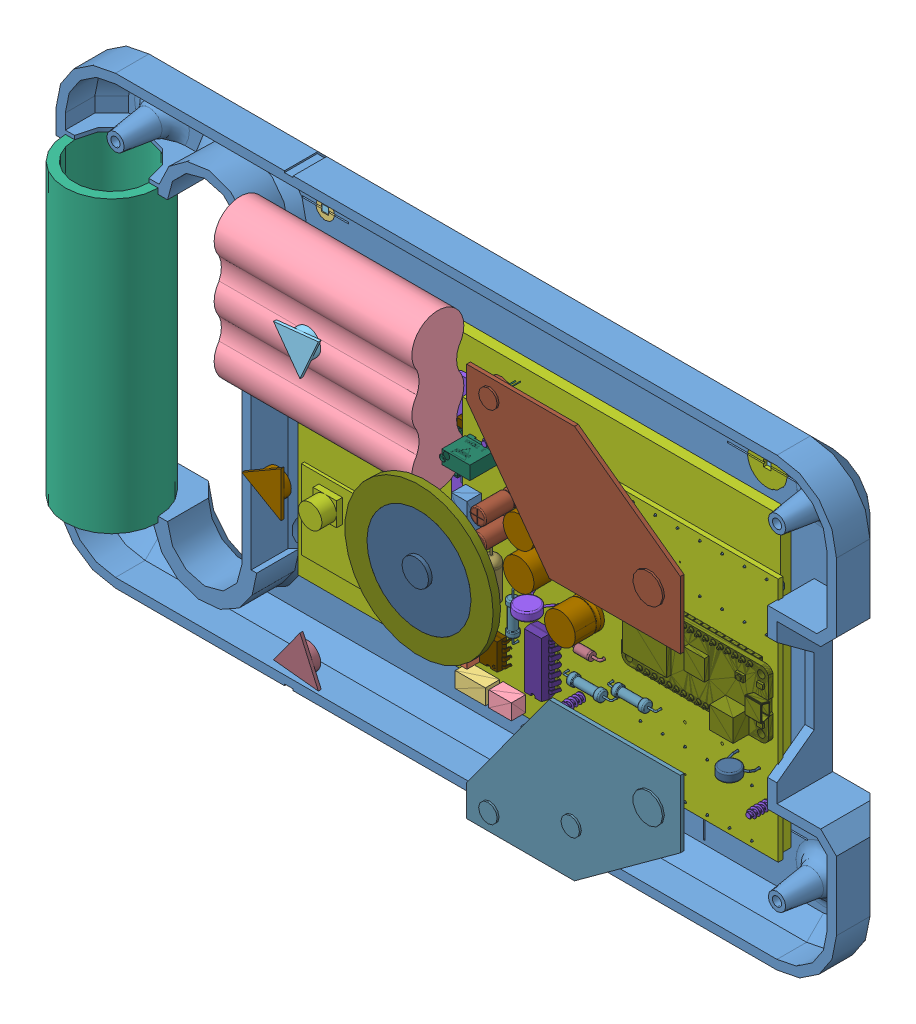
SolidWorks assembly sheikah assembled, configuration Default. Lengths in mm.
Overall size (266.7 152.4 43.32).
174 component instances, 63 part files, 41 mates.
Components (placement in the parent):
- Sheikah Slate Body Converted Assembly-1: Sheikah Slate Body Converted Assembly [Default] at origin size (273.52 152.4 41.91)
  - Front Body-1: Front Body [Default] at origin size (266.7 152.4 21.73)
  - Bottom Right Disk-1: Bottom Right Disk [Default] at origin size (9.21 9.21 0.64)
  - Top Right Blue LED Holder-1: Top Right Blue LED Holder [Default] at origin size (6.31 6.31 3.81)
  - Top Left Disk-1: Top Left Disk [Default] at origin size (7.69 7.69 0.64)
  - Eyelash Orange LED1-1: Eyelash Orange LED1 [Default] at origin size (15.32 14.07 3.54)
  - Handle Tube-1: Handle Tube [Default] at origin size (31.75 99.06 31.75)
  - Top Left Blue LED Holder-2: Top Left Blue LED Holder [Default] at origin size (13.47 13.47 3.81)
  - Bottom Right Blue LED Holder-1: Bottom Right Blue LED Holder [Default] at origin size (14.66 14.66 3.81)
  - Eyelash Orange LED2-3: Eyelash Orange LED2 [Default] at origin size (13.36 15.4 3.54)
  - Inner Neopixel Ring Holder-1: Inner Neopixel Ring Holder [Default] at origin size (35.56 35.56 3.81)
  - Left Orange LED Panel-1: Left Orange LED Panel [Default] at origin size (73.01 49.3 4.45)
  - Bottom Middle Blue LED Holder-1: Bottom Middle Blue LED Holder [Default] at origin size (10.16 10.16 3.81)
  - Eyelash Orange LED3-2: Eyelash Orange LED3 [Default] at origin size (15.32 14.07 3.54)
  - Right Orange LED Panel-1: Right Orange LED Panel [Default] at origin size (73.01 49.3 4.45)
  - Bottom Left Blue LED Holder-1: Bottom Left Blue LED Holder [Default] at origin size (11.44 11.44 3.81)
  - Outer Neopixel Ring Holder-1: Outer Neopixel Ring Holder [Default] at origin size (50.68 50.68 2.54)
  - Back Body-1: Back Body [Default] at origin size (273.52 152.4 34.3) (hidden)
- Neopixel Jewel RGBW-1: Neopixel Jewel RGBW [Default] at (92.2855 47.625 14.545) size (23 23 3.23)
  - Neopixel Jewel RGBW.stp-1: Neopixel Jewel RGBW.stp [Default] at origin size (23 23 3.23)
    - WS2812B-NARROW.stp-1: WS2812B-NARROW.stp [Default] at (0 0 1.6) x (0 -1 0) z (0 0 1) size (5 5.45 1.68)
      - body.stp-1: body.stp [Default] at origin size (5 5 1.6)
      - leads.stp-1: leads.stp [Default] at origin size (4.2 5.45 0.88)
      - processor.stp-1: processor.stp [Default] at origin size (0.8 0.6 0.1)
      - lense.stp-1: lense.stp [Default] at origin size (4 4 0.39)
    - WS2812B-NARROW_1.stp-1: WS2812B-NARROW_1.stp [Default] at (6.9 4 1.6) x (-0.866025 -0.5 0) z (0 0 1) size (5 5.45 1.68)
      - body.stp-1: body.stp [Default] at origin size (5 5 1.6)
      - leads.stp-1: leads.stp [Default] at origin size (4.2 5.45 0.88)
      - processor.stp-1: processor.stp [Default] at origin size (0.8 0.6 0.1)
      - lense.stp-1: lense.stp [Default] at origin size (4 4 0.39)
    - WS2812B-NARROW_2.stp-1: WS2812B-NARROW_2.stp [Default] at (-6.9 4 1.6) x (0.866025 -0.5 0) z (0 0 1) size (5 5.45 1.68)
      - body.stp-1: body.stp [Default] at origin size (5 5 1.6)
      - leads.stp-1: leads.stp [Default] at origin size (4.2 5.45 0.88)
      - processor.stp-1: processor.stp [Default] at origin size (0.8 0.6 0.1)
      - lense.stp-1: lense.stp [Default] at origin size (4 4 0.39)
    - WS2812B-NARROW_3.stp-1: WS2812B-NARROW_3.stp [Default] at (-6.9 -4 1.6) x (0.866025 0.5 0) z (0 0 1) size (5 5.45 1.68)
      - body.stp-1: body.stp [Default] at origin size (5 5 1.6)
      - leads.stp-1: leads.stp [Default] at origin size (4.2 5.45 0.88)
      - processor.stp-1: processor.stp [Default] at origin size (0.8 0.6 0.1)
      - lense.stp-1: lense.stp [Default] at origin size (4 4 0.39)
    - WS2812B-NARROW_4.stp-1: WS2812B-NARROW_4.stp [Default] at (0 8 1.6) x (0 -1 0) z (0 0 1) size (5 5.45 1.68)
      - body.stp-1: body.stp [Default] at origin size (5 5 1.6)
      - leads.stp-1: leads.stp [Default] at origin size (4.2 5.45 0.88)
      - processor.stp-1: processor.stp [Default] at origin size (0.8 0.6 0.1)
      - lense.stp-1: lense.stp [Default] at origin size (4 4 0.39)
    - WS2812B-NARROW_5.stp-1: WS2812B-NARROW_5.stp [Default] at (6.9 -4 1.6) x (-0.866025 0.5 0) z (0 0 1) size (5 5.45 1.68)
      - body.stp-1: body.stp [Default] at origin size (5 5 1.6)
      - leads.stp-1: leads.stp [Default] at origin size (4.2 5.45 0.88)
      - processor.stp-1: processor.stp [Default] at origin size (0.8 0.6 0.1)
      - lense.stp-1: lense.stp [Default] at origin size (4 4 0.39)
    - WS2812B-NARROW_6.stp-1: WS2812B-NARROW_6.stp [Default] at (0 -8.2 1.6) x (0 1 0) z (0 0 1) size (5 5.45 1.68)
      - body.stp-1: body.stp [Default] at origin size (5 5 1.6)
      - leads.stp-1: leads.stp [Default] at origin size (4.2 5.45 0.88)
      - processor.stp-1: processor.stp [Default] at origin size (0.8 0.6 0.1)
      - lense.stp-1: lense.stp [Default] at origin size (4 4 0.39)
    - pcb.stp-1: pcb.stp [Default] at origin size (23 23 1.6)
    - C0603.stp-1: C0603.stp [Default] at (-4.7192 -8.094 1.6) x (-0.5 -0.866025 0) z (0 0 1) size (2.33 0.91 0.82)
    - C0603.stp-2: C0603.stp [Default] at (-4.6 8.1 1.6) x (-0.5 0.866025 0) z (0 0 1) size (2.33 0.91 0.82)
    - C0603.stp-3: C0603.stp [Default] at (4.9743 8.1743 1.6) x (0.707107 0.707107 0) z (0 0 1) size (2.33 0.91 0.82)
    - C0603.stp-4: C0603.stp [Default] at (4.694 -8.0316 1.6) x (0.5 -0.866025 0) z (0 0 1) size (2.33 0.91 0.82)
    - R0603-NO.stp-1: R0603-NO.stp [Default] at (-4.2552 0.1809 1.6) x (0 1 0) z (0 0 1) size (2.31 0.91 0.45)
- NeoPixelRing16-1: NeoPixelRing16 [Default] at (92.2855 47.625 15.58) x (0.587442 0.809266 0) z (0 0 1) size (44 44 2.55)
- HDMI 7po adafruit-2: HDMI 7po adafruit [Défaut] at (101.9311 44.1111 -8.025) x (-1 0 0) z (0 0 -1) size (164.95 100 3.45)
- Adafruit RA8875 TFT Breakout-1: Adafruit RA8875 TFT Breakout [Default] at (73.4911 41.9804 -12.425) size (48.26 40.64 4.01)
  - Adafruit RA8875 TFT Breakout.step-1: Adafruit RA8875 TFT Breakout.step [Default] at origin size (48.26 40.64 4.01)
    - PCB Component.step-1: PCB Component.step [Default] at origin size (48.26 40.64 4.01)
      - Board.step-1: Board.step [Default] at origin size (48.26 40.64 1.57)
      - RA8875.step-1: RA8875.step [Default] at (25.646 17.018 1.57) size (16 16 1.6)
      - 10K.step-1: 10K.step [Default] at (14.47 28.702 1.57) x (-1 0 0) z (0 0 1) size (2 1.25 1)
      - 10K.step-2: 10K.step [Default] at (10.406 11.684 1.57) x (0 1 0) z (0 0 1) size (2 1.25 1)
      - 10K.step-3: 10K.step [Default] at (9.644 14.732 1.57) size (2 1.25 1)
      - 10K.step-4: 10K.step [Default] at (13.581 10.668 1.57) x (-1 0 0) z (0 0 1) size (2 1.25 1)
      - 10K.step-5: 10K.step [Default] at (13.962 20.955 1.57) x (-1 0 0) z (0 0 1) size (2 1.25 1)
      - 10K.step-6: 10K.step [Default] at (36.822 17.272 1.57) size (2 1.25 1)
      - 10K.step-7: 10K.step [Default] at (34.917 9.652 1.57) size (2 1.25 1)
      - 10K.step-8: 10K.step [Default] at (16.248 8.382 1.57) x (-1 0 0) z (0 0 1) size (2 1.25 1)
      - 10K.step-9: 10K.step [Default] at (37.33 23.241 1.57) x (0 -1 0) z (0 0 1) size (2 1.25 1)
      - 10K.step-10: 10K.step [Default] at (12.438 8.382 1.57) x (-1 0 0) z (0 0 1) size (2 1.25 1)
      - 10K.step-11: 10K.step [Default] at (13.962 19.05 1.57) x (-1 0 0) z (0 0 1) size (2 1.25 1)
      - 10K.step-12: 10K.step [Default] at (13.962 17.272 1.57) x (-1 0 0) z (0 0 1) size (2 1.25 1)
      - 10K.step-13: 10K.step [Default] at (36.822 15.113 1.57) size (2 1.25 1)
      - 10K.step-14: 10K.step [Default] at (38.981 10.414 1.57) x (0 1 0) z (0 0 1) size (2 1.25 1)
      - 20MHz.step-1: 20MHz.step [Default] at (13.454 13.716 1.57) x (0 1 0) z (0 0 1) size (3.8 3 0.4)
      - 33.step-1: 33.step [Default] at (31.996 29.21 1.57) size (3.05 1.6 0.5)
      - 33.step-2: 33.step [Default] at (28.186 29.21 1.57) size (3.05 1.6 0.5)
      - 33.step-3: 33.step [Default] at (24.376 29.21 1.57) size (3.05 1.6 0.5)
      - 33.step-4: 33.step [Default] at (20.566 29.21 1.57) size (3.05 1.6 0.5)
      - 33.step-5: 33.step [Default] at (35.806 29.21 1.57) size (3.05 1.6 0.5)
      - 40PINFPCM4-1734839-0.step-1: 40PINFPCM4-1734839-0.step [Default] at (28.44 37.592 1.57) size (25.43 5.11 2.05)
      - FAN5333BSX.step-1: FAN5333BSX.step [Default] at (2.786 21.082 1.57) x (-1 0 0) z (0 0 1) size (3 3 1.4)
      - 3Ω.step-1: 3Ω.step [Default] at (6.596 18.034 1.57) size (2 1.25 0.85)
      - 3Ω.step-2: 3Ω.step [Default] at (2.786 24.13 1.57) x (-1 0 0) z (0 0 1) size (2 1.25 0.85)
      - 3Ω.step-3: 3Ω.step [Default] at (12.962 24.638 1.57) x (0 -1 0) z (0 0 1) size (2 1.25 0.85)
      - 3Ω.step-4: 3Ω.step [Default] at (6.731 25.916 1.57) size (2 1.25 0.85)
      - 3Ω.step-5: 3Ω.step [Default] at (2.786 18.034 1.57) size (2 1.25 0.85)
      - 3Ω.step-6: 3Ω.step [Default] at (17.01 29.972 1.57) x (0 -1 0) z (0 0 1) size (2 1.25 0.85)
      - 3Ω.step-7: 3Ω.step [Default] at (2.278 11.43 1.57) x (0 1 0) z (0 0 1) size (2 1.25 0.85)
      - 3Ω.step-8: 3Ω.step [Default] at (15.559 33.198 1.57) x (-1 0 0) z (0 0 1) size (2 1.25 0.85)
      - 3Ω.step-9: 3Ω.step [Default] at (8.628 11.811 1.57) x (0 1 0) z (0 0 1) size (2 1.25 0.85)
      - 3Ω.step-10: 3Ω.step [Default] at (6.723 8.763 1.57) x (-1 0 0) z (0 0 1) size (2 1.25 0.85)
      - 3Ω.step-11: 3Ω.step [Default] at (2.667 25.908 1.57) size (2 1.25 0.85)
      - 3Ω.step-12: 3Ω.step [Default] at (1.27 29.972 1.57) x (0 1 0) z (0 0 1) size (2 1.25 0.85)
      - 6.8uH large inductor.step-1: 6.8uH large inductor.step [Default] at (7.358 21.844 1.57) x (0 1 0) z (0 0 1) size (4 4 1.8)
      - MBR0540.step-1: MBR0540.step [Default] at (11.168 24.511 1.57) x (0 -1 0) z (0 0 1) size (3.6 1.4 1.35)
      - MM3Z24VT1G.step-1: MM3Z24VT1G.step [Default] at (6.215 28.702 1.57) x (-1 0 0) z (0 0 1) size (5.04 2.7 2.44)
      - MIC5225-3.3v.step-1: MIC5225-3.3v.step [Default] at (5.326 11.684 1.57) x (0 1 0) z (0 0 1) size (3 3 1.4)
      - 74HC4050.step-1: 74HC4050.step [Default] at (43.045 19.685 1.57) x (0 -1 0) z (0 0 1) size (10 6.2 1.75)
      - 1N4148.step-1: 1N4148.step [Default] at (5.842 15.113 1.57) size (2.7 1.35 1.1)
      - 1N4148.step-2: 1N4148.step [Default] at (2.54 15.113 1.57) x (-1 0 0) z (0 0 1) size (2.7 1.35 1.1)
- adafruit 5035 battery-1: adafruit 5035 battery [Default] at (52.8771 89.0109 15.875) x (-1 0 0) z (0 0 -1) size (67.56 53.34 17.78)
- HLMP-QB00-S0000-1: HLMP-QB00-S0000 [Default] at (24.6439 5.2882 -17.526) x (-1 0 0) z (0 0 1) size (2.21 2.21 2.79)
- HLMP-QB00-S0000-2: HLMP-QB00-S0000 [Default] at (119.6309 -5.6441 -17.526) x (-1 0 0) z (0 0 1) size (2.21 2.21 2.79)
- HLMP-QB00-S0000-3: HLMP-QB00-S0000 [Default] at (172.4751 -0.773 -17.525) x (-1 0 0) z (0 0 1) size (2.21 2.21 2.79)
- HLMP-QB00-S0000-4: HLMP-QB00-S0000 [Default] at (176.2779 103.3091 -18.542) x (-1 0 0) z (0 0 1) size (2.21 2.21 2.79)
- HLMP-QB00-S0000-5: HLMP-QB00-S0000 [Default] at (25.225 103.4991 -17.526) x (-1 0 0) z (0 0 1) size (2.21 2.21 2.79)
- SLR-343DC3F-1: SLR-343DC3F [Default] at (169.1626 80.1556 11.38) x (-0.923728 -0.383049 0) z (-0.383049 0.923728 0) size (3.8 9.21 3.51)
- SLR-343DC3F-2: SLR-343DC3F [Default] at (114.5671 -13.6866 11.38) x (-0.923728 -0.383049 0) z (-0.383049 0.923728 0) size (3.8 9.21 3.51)
- SLR-343DC3F-3: SLR-343DC3F [Default] at (142.6962 -3.5762 11.38) x (-0.923728 -0.383049 0) z (-0.383049 0.923728 0) size (3.8 9.21 3.51)
- SLR-343DC3F-4: SLR-343DC3F [Default] at (169.1626 15.0944 11.38) x (-0.923728 -0.383049 0) z (-0.383049 0.923728 0) size (3.8 9.21 3.51)
- SLR-343DC3F-6: SLR-343DC3F [Default] at (114.5671 108.9366 11.38) x (-0.923728 -0.383049 0) z (-0.383049 0.923728 0) size (3.8 9.21 3.51)
- MCB-1: MCB [Default] at (101.2945 92.9812 -3.2654) x (0 -1 0) z (0 0 1) size (83.82 111.16 36.76)
  - SHEIKAHSLATE-1: SHEIKAHSLATE [Default] at origin size (83.82 111.16 36.76)
    - Board_SHEIKAHSLATE-1: Board_SHEIKAHSLATE [Default] at origin size (83.82 107.95 1.59)
    - HAU470KBAUARKR-1: HAU470KBAUARKR [Default] at (53.34 12.7 0.05) x (0 1 0) z (0 0 1) size (8 3 13.01)
    - MALREKA00DE433BG0K-1: MALREKA00DE433BG0K [Default] at (50.8 26.83 0.05) x (0 1 0) z (0 0 1) size (10.51 10.5 11.95)
    - MALREKA00DE433BG0K-2: MALREKA00DE433BG0K [Default] at (29.21 12.7 0.05) size (10.51 10.5 11.95)
    - MALREKA00DE433BG0K-3: MALREKA00DE433BG0K [Default] at (41.91 12.7 0.05) size (10.51 10.5 11.95)
    - A102J15C0GF5UAAP-1: A102J15C0GF5UAAP [Default] at (67.31 81.28 0.05) x (0 -1 0) z (0 0 1) size (7.99 3 12.01)
    - Noname_1-1: Noname_1 [Default] at (36.83 1.27 0.05) size (5.5 5.5 14.5)
    - Noname_1-2: Noname_1 [Default] at (29.21 1.27 0.05) size (5.5 5.5 14.5)
    - TVA1161-1: TVA1161 [Default] at (54.61 -3.81 0.05) size (21.4 5.51 7.51)
    - 1N5819G-1: 1N5819G [Default] at (62.23 26.67 0) x (0 -1 0) z (0 0 1) size (11.27 2.71 4.71)
    - Noname_2-1: Noname_2 [Default] at (67.31 43.18 0) x (0 -1 0) z (0 0 1) size (16.91 3.6 5.6)
    - Noname_2-2: Noname_2 [Default] at (46.99 58.42 -1.5896) x (0 1 0) z (0 0 -1) size (16.91 3.6 5.6)
    - Noname_2-3: Noname_2 [Default] at (19.05 87.63 -1.5896) x (-1 0 0) z (0 0 -1) size (16.91 3.6 5.6)
    - Noname_2-4: Noname_2 [Default] at (19.05 80.01 -1.5896) x (-1 0 0) z (0 0 -1) size (16.91 3.6 5.6)
    - Noname_2-5: Noname_2 [Default] at (19.05 72.39 -1.5896) x (-1 0 0) z (0 0 -1) size (16.91 3.6 5.6)
    - Noname_2-6: Noname_2 [Default] at (19.05 64.77 -1.5896) x (-1 0 0) z (0 0 -1) size (16.91 3.6 5.6)
    - Noname_2-7: Noname_2 [Default] at (19.05 57.15 -1.5896) x (-1 0 0) z (0 0 -1) size (16.91 3.6 5.6)
    - Noname_2-8: Noname_2 [Default] at (19.05 49.53 -1.5896) x (-1 0 0) z (0 0 -1) size (16.91 3.6 5.6)
    - Noname_2-9: Noname_2 [Default] at (19.05 41.91 -1.5896) x (-1 0 0) z (0 0 -1) size (16.91 3.6 5.6)
    - Noname_2-10: Noname_2 [Default] at (19.05 34.29 -1.5896) x (-1 0 0) z (0 0 -1) size (16.91 3.6 5.6)
    - Noname_2-11: Noname_2 [Default] at (19.05 26.67 -1.5896) x (-1 0 0) z (0 0 -1) size (16.91 3.6 5.6)
    - Noname_2-12: Noname_2 [Default] at (19.05 19.05 -1.5896) x (-1 0 0) z (0 0 -1) size (16.91 3.6 5.6)
    - Noname_2-13: Noname_2 [Default] at (82.55 44.45 -1.5896) x (1 0 0) z (0 0 -1) size (16.91 3.6 5.6)
    - Noname_2-14: Noname_2 [Default] at (82.55 52.07 -1.5896) x (1 0 0) z (0 0 -1) size (16.91 3.6 5.6)
    - Noname_2-15: Noname_2 [Default] at (82.55 59.69 -1.5896) x (1 0 0) z (0 0 -1) size (16.91 3.6 5.6)
    - Noname_2-16: Noname_2 [Default] at (82.55 67.31 -1.5896) x (1 0 0) z (0 0 -1) size (16.91 3.6 5.6)
    - Noname_2-17: Noname_2 [Default] at (82.55 74.93 -1.5896) x (1 0 0) z (0 0 -1) size (16.91 3.6 5.6)
    - Noname_2-18: Noname_2 [Default] at (82.55 82.55 -1.5896) x (1 0 0) z (0 0 -1) size (16.91 3.6 5.6)
    - Noname_2-19: Noname_2 [Default] at (48.26 78.74 -1.5896) x (0 -1 0) z (0 0 -1) size (16.91 3.6 5.6)
    - Noname_2-20: Noname_2 [Default] at (39.37 78.74 -1.5896) x (0 1 0) z (0 0 -1) size (16.91 3.6 5.6)
    - Noname_2-21: Noname_2 [Default] at (71.755 27.94 0) x (0 1 0) z (0 0 1) size (16.91 3.6 5.6)
    - Noname_2-22: Noname_2 [Default] at (39.37 58.42 -1.5896) x (0 1 0) z (0 0 -1) size (16.91 3.6 5.6)
    - Noname_2-23: Noname_2 [Default] at (63.5 2.54 0) size (16.91 3.6 5.6)
    - T93YA-1: T93YA [Default] at (20.32 -13.69 5) size (12.52 14.14 22.04)
    - Adafruit_Feather_M0_Adalogger-1: Adafruit_Feather_M0_Adalogger [Default] at (45.72 66.04 3) x (0 -1 0) z (0 0 1) size (54.99 41.16 36.76)
    - SN74HC125N-1: SN74HC125N [Default] at (71.24 12.69 0) x (-1 0 0) z (0 1 0) size (19.31 8.27 10.93)
    - DIP8-1: DIP8 [Default] at (76.2 -3.81 0) size (15.36 12.48 12.48)
    - DIP8-2: DIP8 [Default] at (35.77 29 0) x (0 1 0) z (0 0 1) size (15.36 12.48 12.48)
    - 640453-4-1: 640453-4 [Default] at (39.1318 -16.4465 0) size (10.3 5.34 4.91)
    - 1-640453-5-1: 1-640453-5 [Default] at (64.53 -16.4465 0) size (38.24 5.34 4.91)
    - 640453-4-0-1: 640453-4-0 [Default] at (92.6465 -9.1282 0) x (0 1 0) z (0 0 1) size (10.3 5.34 4.91)
    - 640453-3-1: 640453-3 [Default] at (92.6465 1.0303 0) x (-0.000018 1 0) z (0 0 1) size (7.76 5.34 4.91)
    - PPTC021LFBN-RC-1: PPTC021LFBN-RC [Default] at (88.689 15.24 0) x (0 1 0) z (0 0 1) size (5.94 2.66 8.76)
    - PPTC021LFBN-RC-1-1: PPTC021LFBN-RC-1 [Default] at (88.689 24.13 0) x (-0.000018 1 0) z (0 0 1) size (5.94 2.66 8.76)
- adafruit TTL mini camera-1: adafruit TTL mini camera [Default] at (57.6381 41.125 14.59) x (-1 0 0) z (0 0 -1) size (20 27 14)
- 99461A941_Phillips Rounded Head Thread-Forming Screws-1: 99461A941_Phillips Rounded Head Thread-Forming Screws [99461A941] at (-30.48 -8.255 -12.2325) x (-0.923728 -0.383049 0) z (0 0 -1) size (5.3 5.3 10.3)
- 99461A941_Phillips Rounded Head Thread-Forming Screws-2: 99461A941_Phillips Rounded Head Thread-Forming Screws [99461A941] at (195.58 -8.255 -12.2325) x (-0.923728 -0.383049 0) z (0 0 -1) size (5.3 5.3 10.3)
- 99461A941_Phillips Rounded Head Thread-Forming Screws-3: 99461A941_Phillips Rounded Head Thread-Forming Screws [99461A941] at (-30.48 103.505 -12.2325) x (-0.923728 -0.383049 0) z (0 0 -1) size (5.3 5.3 10.3)
- 99461A941_Phillips Rounded Head Thread-Forming Screws-4: 99461A941_Phillips Rounded Head Thread-Forming Screws [99461A941] at (195.58 103.505 -12.2325) x (-0.923728 -0.383049 0) z (0 0 -1) size (5.3 5.3 10.3)
- 99461A941_Phillips Rounded Head Thread-Forming Screws-5: 99461A941_Phillips Rounded Head Thread-Forming Screws [99461A941] at (98.7545 80.2812 -4.6875) x (-0.923728 -0.383049 0) z (0 0 -1) size (5.3 5.3 10.3)
- 99461A941_Phillips Rounded Head Thread-Forming Screws-6: 99461A941_Phillips Rounded Head Thread-Forming Screws [99461A941] at (125.4245 15.5112 -4.6875) x (-0.923728 -0.383049 0) z (0 0 -1) size (5.3 5.3 10.3)
- 99461A941_Phillips Rounded Head Thread-Forming Screws-7: 99461A941_Phillips Rounded Head Thread-Forming Screws [99461A941] at (189.0345 15.5112 -4.6875) x (-0.923728 -0.383049 0) z (0 0 -1) size (5.3 5.3 10.3)
Mates (geometry in assembly coordinates):
- Coincident10: coincident: plane of HDMI 7po adafruit-2 through (184.4061 94.1111 -12.425) normal (0 0 1); plane of Adafruit RA8875 TFT Breakout-1/Adafruit RA8875 TFT Breakout.step-1/PCB Component.step-1/Board.step-1 through (97.6211 62.3004 -12.425) normal (0 0 -1)
- Coincident11: coincident: plane of HDMI 7po adafruit-2 through (101.9311 44.1111 -8.025) normal (-1 0 0); moEndPointRef_w of Adafruit RA8875 TFT Breakout-1/Adafruit RA8875 TFT Breakout.step-1/PCB Component.step-1/40PINFPCM4-1734839-0.step-1
- Parallel2: parallel aligned: line of HDMI 7po adafruit-2 through (184.4061 94.1111 -12.425) axis (0 -1 0); line of Adafruit RA8875 TFT Breakout-1/Adafruit RA8875 TFT Breakout.step-1/PCB Component.step-1/Board.step-1 through (121.7511 80.0804 -12.425) axis (0 -1 0)
- Coincident13: coincident: plane of sheikah slate-1 through (0 95.25 15.875) normal (0 0 -1); plane of adafruit 5035 battery-1 through (52.8771 89.0109 15.875) normal (0 0 -1)
- Coincident14: coincident anti-aligned: plane of sheikah slate-1 through (0 95.25 15.875) normal (0 0 -1); plane of Adafruit MicroUSB Micro Lipo-1 through (192.405 6.2327 15.875) normal (0 0 1)
- Coincident15: coincident anti-aligned: plane of sheikah slate-1 through (192.405 20.6375 19.05) normal (-1 0 0); plane of Adafruit MicroUSB Micro Lipo-1 through (192.405 6.2327 15.875) normal (1 0 0)
- Coincident20: coincident: plane of sheikah slate-1 through (25.7489 6.5832 -18.796) normal (-1 0 0); plane of HLMP-QB00-S0000-1 through (25.7489 4.1832 -16.002) normal (1 0 0)
- Coincident21: coincident: plane of sheikah slate-1 through (23.3489 4.1832 -18.796) normal (0 1 0); plane of HLMP-QB00-S0000-1 through (25.7489 4.1832 -16.002) normal (0 -1 0)
- Coincident22: coincident: plane of sheikah slate-1 through (0 0 -18.796) normal (0 0 1); circle of HLMP-QB00-S0000-1
- Coincident23: coincident: plane of sheikah slate-1 through (118.5259 -6.7491 -18.796) normal (0 1 0); plane of HLMP-QB00-S0000-2 through (120.7359 -6.7491 -16.002) normal (0 -1 0)
- Coincident24: coincident: plane of sheikah slate-1 through (118.5259 -4.3491 -18.796) normal (1 0 0); plane of HLMP-QB00-S0000-2 through (118.5259 -6.7491 -16.002) normal (-1 0 0)
- Coincident25: coincident: plane of sheikah slate-1 through (0 0 -18.796) normal (0 0 1); circle of HLMP-QB00-S0000-2
- Coincident26: coincident: plane of sheikah slate-1 through (171.1801 -1.878 -18.795) normal (0 1 0); plane of HLMP-QB00-S0000-3 through (173.5801 -1.878 -16.001) normal (0 -1 0)
- Coincident27: coincident: plane of sheikah slate-1 through (173.5801 0.522 -18.795) normal (-1 0 0); plane of HLMP-QB00-S0000-3 through (173.5801 -1.878 -16.001) normal (1 0 0)
- Tangent1: tangent: plane of sheikah slate-1 through (0 0 -18.795) normal (0 0 1); torus of HLMP-QB00-S0000-3
- Coincident28: coincident: plane of sheikah slate-1 through (175.1729 102.2041 -18.796) normal (0 1 0); plane of HLMP-QB00-S0000-4 through (177.3829 102.2041 -17.018) normal (0 -1 0)
- Coincident29: coincident: plane of sheikah slate-1 through (175.1729 104.6041 -18.796) normal (1 0 0); plane of HLMP-QB00-S0000-4 through (175.1729 102.2041 -17.018) normal (-1 0 0)
- Tangent2: tangent: plane of sheikah slate-1 through (0 0 -18.796) normal (0 0 1); torus of HLMP-QB00-S0000-4
- Coincident30: coincident: plane of sheikah slate-1 through (24.12 104.6041 -18.796) normal (1 0 0); plane of HLMP-QB00-S0000-5 through (24.12 102.3941 -16.002) normal (-1 0 0)
- Coincident31: coincident: plane of sheikah slate-1 through (24.12 104.6041 -18.796) normal (0 -1 0); plane of HLMP-QB00-S0000-5 through (26.33 104.6041 -16.002) normal (0 1 0)
- Coincident32: coincident: plane of sheikah slate-1 through (0 0 -18.796) normal (0 0 1); plane of HLMP-QB00-S0000-5 through (25.225 103.4991 -18.796) normal (0 0 -1)
- Concentric3: concentric: cylinder of sheikah slate-1 through (169.1626 80.1556 23.2247) axis (0 0 -1) radius 1.925; cylinder of SLR-343DC3F-1 through (169.1626 80.1556 16.78) axis (0 0 -1) radius 1.9
- Coincident34: coincident: plane of sheikah slate-1 through (0 95.25 16.78) normal (0 0 -1); circle of SLR-343DC3F-1
- Coincident35: coincident: plane of sheikah slate-1 through (192.405 20.6375 19.05) normal (-1 0 0); plane of MCB-1/SHEIKAHSLATE^MCB-1/Board_SHEIKAHSLATE^SHEIKAHSLATE_MCB-1 through (192.405 0.7596 -3.2654) normal (1 0 0)
- Distance1: distance = 6 mm: plane of MCB-1/SHEIKAHSLATE^MCB-1/Board_SHEIKAHSLATE^SHEIKAHSLATE_MCB-1 through (84.7845 84.0912 -4.855) normal (0 0 -1); plane of Adafruit RA8875 TFT Breakout-1/Adafruit RA8875 TFT Breakout.step-1/PCB Component.step-1/Board.step-1 through (97.6211 62.3004 -10.855) normal (0 0 1)
- Coincident37: coincident: plane of sheikah slate-1 through (54.1619 47.625 19.05) normal (0 -1 0); plane of MCB-1/SHEIKAHSLATE-1 through (100.965 47.625 -3.2654) normal (0 1 0)
- Parallel3: parallel: line of sheikah slate-1 through (106.6802 114.8899 15.875) axis (-1 0 0); line of adafruit 5035 battery-1 through (86.6591 101.583 -0.2198) axis (-1 0 0)
- Coincident39: coincident: line of sheikah slate-1 through (19.0951 95.25 15.875) axis (0 -1 0); plane of adafruit 5035 battery-1 through (19.0951 116.9509 -1.905) normal (-1 0 0)
- Coincident41: coordinate: unknown of sheikah slate-2
- Concentric4: concentric aligned: circle of Sheikah Slate Body Converted Assembly-1/Back Body-1; circle of adafruit TTL mini camera-1
- Parallel4: parallel anti-aligned: line of Sheikah Slate Body Converted Assembly-1/Back Body-1 through (47.6381 28.625 15.875) axis (1 0 0); line of adafruit TTL mini camera-1 through (67.6381 27.625 14.59) axis (-1 0 0)
- Coincident43: coincident aligned: plane of Sheikah Slate Body Converted Assembly-1/Back Body-1 through (0 0 21.59) normal (0 0 1); plane of adafruit TTL mini camera-1 through (57.6381 47.625 21.59) normal (0 0 1)
- Concentric5: concentric anti-aligned: circle of Sheikah Slate Body Converted Assembly-1/Front Body-1; circle of 99461A941_Phillips Rounded Head Thread-Forming Screws-1
- Coincident45: coincident aligned: plane of Sheikah Slate Body Converted Assembly-1/Front Body-1 through (-28.88 -8.255 -12.4) normal (0 0 -1); circle of 99461A941_Phillips Rounded Head Thread-Forming Screws-1
- Concentric6: concentric aligned: circle of MCB-1/SHEIKAHSLATE-1/Board_SHEIKAHSLATE-1; circle of 99461A941_Phillips Rounded Head Thread-Forming Screws-5
- Coincident46: coincident: plane of MCB-1/SHEIKAHSLATE-1/Board_SHEIKAHSLATE-1 through (84.7845 84.0912 -4.855) normal (0 0 -1); circle of 99461A941_Phillips Rounded Head Thread-Forming Screws-5
- Concentric8: concentric: circle of Sheikah Slate Body Converted Assembly-1/Back Body-1; circle of 99461A941_Phillips Rounded Head Thread-Forming Screws-5
- Coincident48: coincident: circle of Sheikah Slate Body Converted Assembly-1/Back Body-1; plane of MCB-1/SHEIKAHSLATE-1/Board_SHEIKAHSLATE-1 through (84.7845 84.0912 -3.2654) normal (0 0 1)
- Parallel6: parallel: line of Sheikah Slate Body Converted Assembly-1/Back Body-1 through (26.5 192.405 51.2875) axis (0 0 1); plane of MCB-1/SHEIKAHSLATE-1/Board_SHEIKAHSLATE-1 through (192.7345 0.2712 -3.2654) normal (1 0 0)
- Coincident53: coincident anti-aligned: line of Sheikah Slate Body Converted Assembly-1/Front Body-1 through (31.6784 1.6111 -15.875) axis (1 0 0); line of HDMI 7po adafruit-2 through (181.7861 1.6111 -15.875) axis (-1 0 0)
- Coincident54: coincident anti-aligned: line of Sheikah Slate Body Converted Assembly-1/Front Body-1 through (25.2861 87.5111 -15.875) axis (0 -1 0); line of HDMI 7po adafruit-2 through (25.2861 1.6111 -15.875) axis (0 1 0)
